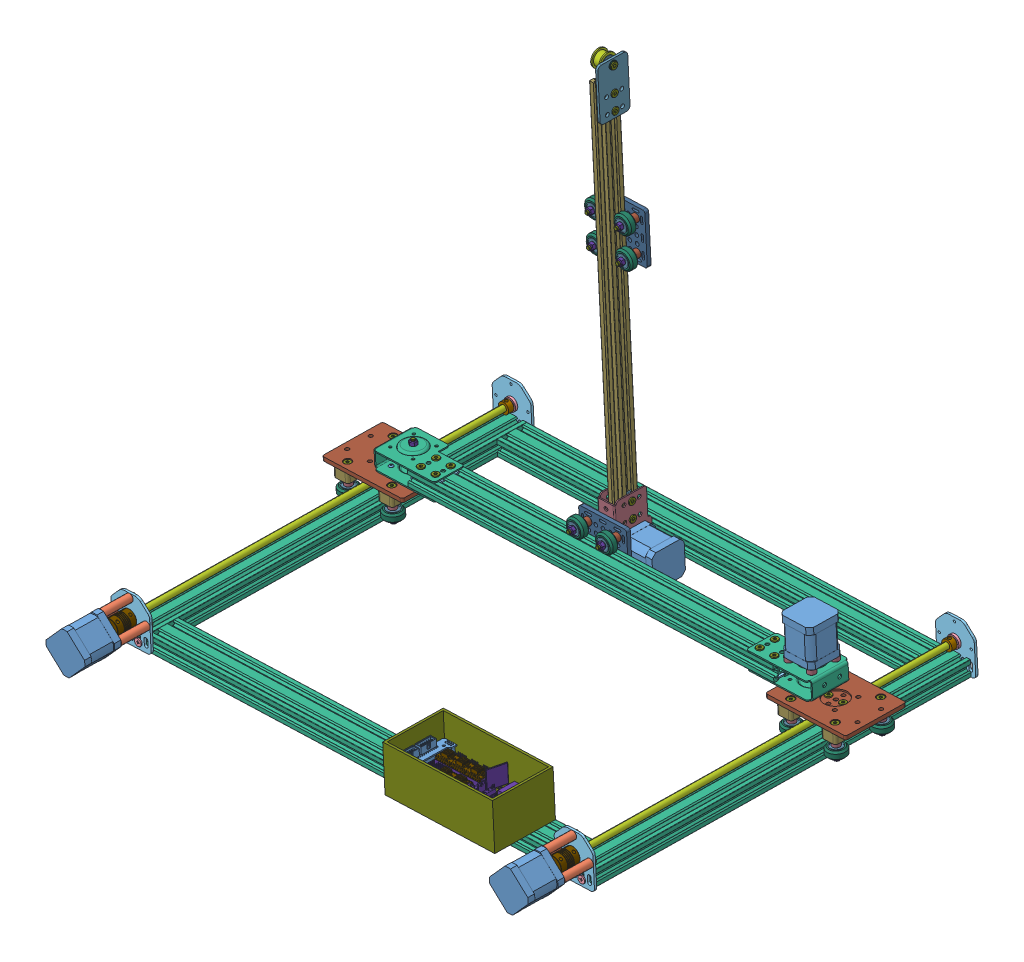
SolidWorks assembly manipulator2, configuration 預設. Lengths in mm.
Overall size (716.52 632.46 604.45).
279 component instances, 37 part files, 37 mates.
Components (placement in the parent):
- Button Head Socket Cap Screw M3-1: Button Head Socket Cap Screw M3 [M3 x 17] at (-19.1837 8.1538 443.4891) x (0.052967 -0.998596 -0.000534) z (0.000534 -0.000506 1) size (18.72 5.7 5.7)
- Button Head Socket Cap Screw M3-2: Button Head Socket Cap Screw M3 [M3 x 17] at (11.7683 9.7952 444.0184) x (0.052967 -0.998596 -0.000534) z (0.000534 -0.000506 1) size (18.72 5.7 5.7)
- Button Head Socket Cap Screw M3-3: Button Head Socket Cap Screw M3 [M3 x 17] at (-19.7114 8.1092 474.4845) x (0.052967 -0.998596 -0.000534) z (0.000534 -0.000506 1) size (18.72 5.7 5.7)
- Button Head Socket Cap Screw M3-4: Button Head Socket Cap Screw M3 [M3 x 17] at (11.2406 9.7507 475.0139) x (0.052967 -0.998596 -0.000534) z (0.000534 -0.000506 1) size (18.72 5.7 5.7)
- Nylon Insert Lock Nut M3-3: Nylon Insert Lock Nut M3 [Default] at (11.5352 14.189 444.0207) x (-0.998393 -0.052967 0.02015) z (0.02015 0.000534 0.999797) size (5.5 4 6.35)
- Nylon Insert Lock Nut M3-4: Nylon Insert Lock Nut M3 [Default] at (11.0075 14.1445 475.0162) x (-0.998393 -0.052967 0.02015) z (0.02015 0.000534 0.999797) size (5.5 4 6.35)
- Nylon Insert Lock Nut M3-5: Nylon Insert Lock Nut M3 [Default] at (-19.9445 12.503 474.4869) x (-0.998393 -0.052967 0.02015) z (0.02015 0.000534 0.999797) size (5.5 4 6.35)
- Nylon Insert Lock Nut M3-6: Nylon Insert Lock Nut M3 [Default] at (-19.4168 12.5476 443.4914) x (-0.998393 -0.052967 0.02015) z (0.02015 0.000534 0.999797) size (5.5 4 6.35)
- Aluminum Spacer 3mm-1: Aluminum Spacer 3mm [6mm] at (10.9526 25.1736 444.0266) x (0.997193 0.05292 -0.052967) z (0.052967 -0.998596 -0.000534) size (10 10 6)
- Aluminum Spacer 3mm-2: Aluminum Spacer 3mm [6mm] at (-19.9994 23.5322 443.4973) x (0.997193 0.05292 -0.052967) z (0.052967 -0.998596 -0.000534) size (10 10 6)
- Aluminum Spacer 3mm-3: Aluminum Spacer 3mm [6mm] at (-20.5271 23.4876 474.4928) x (0.997193 0.05292 -0.052967) z (0.052967 -0.998596 -0.000534) size (10 10 6)
- Aluminum Spacer 3mm-4: Aluminum Spacer 3mm [6mm] at (10.4249 25.129 475.0221) x (0.997193 0.05292 -0.052967) z (0.052967 -0.998596 -0.000534) size (10 10 6)
- Z2-1: Z2 [Default] at (-565.1545 -15.5578 336.9084) size (111.46 63.72 594.1) (flexible)
  - Ball Bearing 8 x 16 x 5-4: Ball Bearing 8 x 16 x 5 [Default] at (533.6792 21.533 -34.6863) x (-0.017023 -0.001438 0.999854) z (-0.57924 -0.815083 -0.011034) size (5 16 16)
  - Threaded Rod Plate Nema 17-3: Threaded Rod Plate Nema 17 [Default] at (533.7388 21.538 -38.1858) x (0.998451 0.05295 0.017075) z (0.052967 -0.998596 -0.000534) size (53 3 59.29)
  - V-Slot 20x40x500 Linear Rail-1: V-Slot 20x40x500 Linear Rail [Default] at (534.8758 -0.8648 -35.1982) x (0.052967 -0.998596 -0.000534) z (-0.017023 -0.001438 0.999854) size (20 40 500)
  - Threaded Rod Plate Nema 17-6: Threaded Rod Plate Nema 17 [Default] at (525.1253 20.8106 467.7404) x (-0.998451 -0.05295 -0.017075) z (0.052967 -0.998596 -0.000534) size (53 3 59.29)
  - Ball Bearing 8 x 16 x 5-6: Ball Bearing 8 x 16 x 5 [Default] at (525.1849 20.8156 464.2409) x (0.017023 0.001438 -0.999854) z (0.999854 0.001413 0.017025) size (5 16 16)
  - 8mm leadscrew 540mm-1: 8mm leadscrew 540mm [520mm] at (533.7388 21.538 -38.1858) x (-0.290929 0.956738 -0.003577) z (-0.017023 -0.001438 0.999854) size (8 8 520)
  - Shim Washer 8mm-5: Shim Washer 8mm [Default] at (525.2274 20.8192 461.7412) x (0.999711 -0.017023 0.016996) z (0.016996 0.999854 0.001727) size (11.8 1.15 11.8)
  - Shim Washer 8mm-6: Shim Washer 8mm [Default] at (533.6367 21.5294 -32.1867) x (0.99971 0.017023 0.017045) z (0.017045 -0.999854 -0.001147) size (11.8 1.15 11.8)
  - Lock Collar 8mm-5: Lock Collar 8mm [Default] at (525.3662 20.8309 453.5924) x (0.999855 -0.000012 0.017023) z (-0.017023 -0.001438 0.999854) size (14 14 7)
  - Lock Collar 8mm-6: Lock Collar 8mm [Default] at (533.6171 21.5277 -31.0369) x (0.999855 -0.000012 0.017023) z (-0.017023 -0.001438 0.999854) size (14 14 7)
  - 8mm Acme Nut Block-3: 8mm Acme Nut Block [Default] at (531.1848 21.3223 111.8263) x (-0.998451 -0.05295 -0.017075) z (-0.017023 -0.001438 0.999854) size (34 12 20)
  - mid plate-3: mid plate [預設] at (528.4577 31.3097 -5.2228) x (0.998451 0.05295 0.017075) z (-0.017023 -0.001438 0.999854) size (110 42 86.72)
    - V-Slot Gantry Plate 20-80mm 2-1: V-Slot Gantry Plate 20-80mm 2 [Default] at (4.1926 -4.0553 127) size (110 5 80)
    - Spacer Block 2-1: Spacer Block 2 [Default] at (-26.1074 -16.0553 127) x (0 0 -1) z (0 1 0) size (80 20 12)
    - Spacer Block 2-2: Spacer Block 2 [Default] at (34.4926 -16.0553 127) x (0 0 -1) z (0 1 0) size (80 20 12)
    - Aluminum Spacer 6mm-1: Aluminum Spacer 6mm [9mm] at (34.4926 -25.0553 97) x (1 0 0) z (0 1 0) size (10 10 9)
    - Aluminum Spacer 6mm-2: Aluminum Spacer 6mm [9mm] at (34.4926 -25.0553 157) x (1 0 0) z (0 1 0) size (10 10 9)
    - Aluminum Spacer 6mm-3: Aluminum Spacer 6mm [9mm] at (-26.1074 -25.0553 97) x (1 0 0) z (0 1 0) size (10 10 9)
    - Aluminum Spacer 6mm-4: Aluminum Spacer 6mm [9mm] at (-26.1074 -25.0553 157) x (1 0 0) z (0 1 0) size (10 10 9)
    - small wheel-9: small wheel [預設] at (-14.754 -38.612 99.7479) x (0 -1 0) z (0 0 1) size (11 23.9 23.9)
      - Ball Bearing 5 x 16 x 5-2: Ball Bearing 5 x 16 x 5 [Default] at (-5.0567 -11.3534 -2.7479) size (5 16 16)
      - Solid V Wheel-2: Solid V Wheel [Default] at (-8.0567 -11.3534 -2.7479) size (10.2 23.9 23.9)
      - Ball Bearing 5 x 16 x 5-3: Ball Bearing 5 x 16 x 5 [Default] at (-11.0567 -11.3534 -2.7479) size (5 16 16)
    - small wheel-10: small wheel [預設] at (-14.4269 -38.612 156.8676) x (0 -1 0) z (0.246245 0 0.969207) size (11 23.9 23.9)
      - Ball Bearing 5 x 16 x 5-2: Ball Bearing 5 x 16 x 5 [Default] at (-5.0567 -11.3534 -2.7479) size (5 16 16)
      - Solid V Wheel-2: Solid V Wheel [Default] at (-8.0567 -11.3534 -2.7479) size (10.2 23.9 23.9)
      - Ball Bearing 5 x 16 x 5-3: Ball Bearing 5 x 16 x 5 [Default] at (-11.0567 -11.3534 -2.7479) size (5 16 16)
    - small wheel-11: small wheel [預設] at (46.169 -38.612 156.6628) x (0 -1 0) z (0.263197 0 0.964742) size (11 23.9 23.9)
      - Ball Bearing 5 x 16 x 5-2: Ball Bearing 5 x 16 x 5 [Default] at (-5.0567 -11.3534 -2.7479) size (5 16 16)
      - Solid V Wheel-2: Solid V Wheel [Default] at (-8.0567 -11.3534 -2.7479) size (10.2 23.9 23.9)
      - Ball Bearing 5 x 16 x 5-3: Ball Bearing 5 x 16 x 5 [Default] at (-11.0567 -11.3534 -2.7479) size (5 16 16)
    - small wheel-12: small wheel [預設] at (45.8243 -38.612 99.8362) x (0 -1 0) z (-0.007785 0 0.99997) size (11 23.9 23.9)
      - Ball Bearing 5 x 16 x 5-2: Ball Bearing 5 x 16 x 5 [Default] at (-5.0567 -11.3534 -2.7479) size (5 16 16)
      - Solid V Wheel-2: Solid V Wheel [Default] at (-8.0567 -11.3534 -2.7479) size (10.2 23.9 23.9)
      - Ball Bearing 5 x 16 x 5-3: Ball Bearing 5 x 16 x 5 [Default] at (-11.0567 -11.3534 -2.7479) size (5 16 16)
    - Low Profile Screw M5-6: Low Profile Screw M5 [M5 x 40] at (-26.1074 -41.0553 157) x (0 -1 0) z (0 0 1) size (41.62 9 9)
    - Low Profile Screw M5-7: Low Profile Screw M5 [M5 x 40] at (-26.1074 -41.0553 97) x (0 -1 0) z (0 0 1) size (41.62 9 9)
    - Low Profile Screw M5-8: Low Profile Screw M5 [M5 x 40] at (34.4926 -41.0553 97) x (0 -1 0) z (0 0 1) size (41.62 9 9)
    - Low Profile Screw M5-10: Low Profile Screw M5 [M5 x 40] at (34.4926 -41.0553 157) x (0 -1 0) z (0 0 1) size (41.62 9 9)
    - Nylon Insert Lock Nut M5-5: Nylon Insert Lock Nut M5 [Default] at (-26.1074 -36.0553 157) x (0.837169 0 0.546944) z (0.546944 0 -0.837169) size (8 5 9.24)
    - Nylon Insert Lock Nut M5-6: Nylon Insert Lock Nut M5 [Default] at (-26.1074 -36.0553 97) x (0.837169 0 0.546944) z (0.546944 0 -0.837169) size (8 5 9.24)
    - Nylon Insert Lock Nut M5-7: Nylon Insert Lock Nut M5 [Default] at (34.4926 -36.0553 157) x (0.837169 0 0.546944) z (0.546944 0 -0.837169) size (8 5 9.24)
    - Nylon Insert Lock Nut M5-8: Nylon Insert Lock Nut M5 [Default] at (34.4926 -36.0553 97) x (0.837169 0 0.546944) z (0.546944 0 -0.837169) size (8 5 9.24)
  - Flexible Coupling 5mm x 8mm-4: Flexible Coupling 5mm x 8mm [Default] at (524.6742 20.7725 494.2365) x (-0.433195 0.90128 -0.006079) z (-0.017023 -0.001438 0.999854) size (21.03 20 25)
  - Nema 17 Stepper Motor-3: Nema 17 Stepper Motor [Default] at (524.4784 20.7559 505.7348) x (-0.743465 0.668673 -0.011696) z (0.017023 0.001438 -0.999854) size (42.42 42.42 72)
  - Aluminum Spacer 40mm-5: Aluminum Spacer 40mm [38] at (546.3648 21.9166 506.1091) x (-0.985691 -0.1677 -0.017023) z (0.017023 0.001438 -0.999854) size (10 10 38)
  - Aluminum Spacer 40mm-6: Aluminum Spacer 40mm [38] at (523.3174 42.6455 505.7465) x (-0.985691 -0.1677 -0.017023) z (0.017023 0.001438 -0.999854) size (10 10 38)
  - Aluminum Spacer 40mm-7: Aluminum Spacer 40mm [38] at (502.5921 19.5953 505.3605) x (-0.985691 -0.1677 -0.017023) z (0.017023 0.001438 -0.999854) size (10 10 38)
  - Socket Head Cap Screw M3-8: Socket Head Cap Screw M3 [M3 x 45] at (523.2493 42.6397 509.7459) x (-0.017023 -0.001438 0.999854) z (-0.999854 0.001462 -0.017021) size (48.09 5.5 5.5)
  - Socket Head Cap Screw M3-9: Socket Head Cap Screw M3 [M3 x 45] at (502.524 19.5895 509.3599) x (-0.017023 -0.001438 0.999854) z (-0.999854 0.001462 -0.017021) size (48.09 5.5 5.5)
  - Socket Head Cap Screw M3-10: Socket Head Cap Screw M3 [M3 x 45] at (546.2967 21.9109 510.1085) x (-0.017023 -0.001438 0.999854) z (-0.999854 0.001462 -0.017021) size (48.09 5.5 5.5)
  - Self Tapping Screw-1: Self Tapping Screw [Default] at (536.371 -2.4365 467.8984) x (0.99971 0.017023 0.017045) z (0.017045 -0.999854 -0.001147) size (9.6 20.4 9.6)
  - Self Tapping Screw-2: Self Tapping Screw [Default] at (516.4019 -3.4955 467.5569) x (0.99971 0.017023 0.017045) z (0.017045 -0.999854 -0.001147) size (9.6 20.4 9.6)
  - Self Tapping Screw-3: Self Tapping Screw [Default] at (544.9844 -1.7091 -38.0278) x (0.999711 -0.017023 0.016996) z (0.016996 0.999854 0.001727) size (9.6 20.4 9.6)
  - Self Tapping Screw-4: Self Tapping Screw [Default] at (525.0154 -2.7681 -38.3693) x (0.999711 -0.017023 0.016996) z (0.016996 0.999854 0.001727) size (9.6 20.4 9.6)
  - Nylon Insert Lock Nut M5-1: Nylon Insert Lock Nut M5 [Default] at (541.0521 20.8388 121.9951) x (-0.998393 -0.052967 0.02015) z (0.02015 0.000534 0.999797) size (8 5 9.24)
  - Nylon Insert Lock Nut M5-2: Nylon Insert Lock Nut M5 [Default] at (521.083 19.7798 121.6536) x (-0.998393 -0.052967 0.02015) z (0.02015 0.000534 0.999797) size (8 5 9.24)
  - Low Profile Screw M5-1: Low Profile Screw M5 [M5 x 15] at (541.3169 15.8459 121.9924) x (0.052967 -0.998596 -0.000534) z (0.000534 -0.000506 1) size (16.62 9 9)
  - Low Profile Screw M5-2: Low Profile Screw M5 [M5 x 15] at (521.3479 14.7869 121.6509) x (0.052967 -0.998596 -0.000534) z (0.000534 -0.000506 1) size (16.62 9 9)
- V-Slot 20x40x500 Linear Rail-1: V-Slot 20x40x500 Linear Rail [20 x 40 x 566] at (554.3834 14.5723 331.7116) x (-0.052967 0.998596 0.000534) z (-0.998451 -0.05295 -0.017075) size (20 40 565.91)
- V-Slot 20x40x500 Linear Rail-2: V-Slot 20x40x500 Linear Rail [20 x 40 x 566] at (546.5529 13.911 791.6445) x (-0.052967 0.998596 0.000534) z (-0.998451 -0.05295 -0.017075) size (20 40 565.91)
- Z2-4: Z2 [Default] at (39.9069 16.5297 347.2558) size (111.46 63.72 594.1) (flexible)
  - Ball Bearing 8 x 16 x 5-4: Ball Bearing 8 x 16 x 5 [Default] at (533.6792 21.533 -34.6863) x (-0.017023 -0.001438 0.999854) z (-0.57924 -0.815083 -0.011034) size (5 16 16)
  - Threaded Rod Plate Nema 17-3: Threaded Rod Plate Nema 17 [Default] at (533.7388 21.538 -38.1858) x (0.998451 0.05295 0.017075) z (0.052967 -0.998596 -0.000534) size (53 3 59.29)
  - V-Slot 20x40x500 Linear Rail-1: V-Slot 20x40x500 Linear Rail [Default] at (534.8758 -0.8648 -35.1982) x (0.052967 -0.998596 -0.000534) z (-0.017023 -0.001438 0.999854) size (20 40 500)
  - Threaded Rod Plate Nema 17-6: Threaded Rod Plate Nema 17 [Default] at (525.1253 20.8106 467.7404) x (-0.998451 -0.05295 -0.017075) z (0.052967 -0.998596 -0.000534) size (53 3 59.29)
  - Ball Bearing 8 x 16 x 5-6: Ball Bearing 8 x 16 x 5 [Default] at (525.1849 20.8156 464.2409) x (0.017023 0.001438 -0.999854) z (0.999854 0.001413 0.017025) size (5 16 16)
  - 8mm leadscrew 540mm-1: 8mm leadscrew 540mm [520mm] at (533.7388 21.538 -38.1858) x (-0.290929 0.956738 -0.003577) z (-0.017023 -0.001438 0.999854) size (8 8 520)
  - Shim Washer 8mm-5: Shim Washer 8mm [Default] at (525.2274 20.8192 461.7412) x (0.999711 -0.017023 0.016996) z (0.016996 0.999854 0.001727) size (11.8 1.15 11.8)
  - Shim Washer 8mm-6: Shim Washer 8mm [Default] at (533.6367 21.5294 -32.1867) x (0.99971 0.017023 0.017045) z (0.017045 -0.999854 -0.001147) size (11.8 1.15 11.8)
  - Lock Collar 8mm-5: Lock Collar 8mm [Default] at (525.3662 20.8309 453.5924) x (0.999855 -0.000012 0.017023) z (-0.017023 -0.001438 0.999854) size (14 14 7)
  - Lock Collar 8mm-6: Lock Collar 8mm [Default] at (533.6171 21.5277 -31.0369) x (0.999855 -0.000012 0.017023) z (-0.017023 -0.001438 0.999854) size (14 14 7)
  - 8mm Acme Nut Block-3: 8mm Acme Nut Block [Default] at (531.1848 21.3223 111.8263) x (-0.998451 -0.05295 -0.017075) z (-0.017023 -0.001438 0.999854) size (34 12 20)
  - mid plate-3: mid plate [預設] at (528.4577 31.3097 -5.2228) x (0.998451 0.05295 0.017075) z (-0.017023 -0.001438 0.999854) size (110 42 86.72)
    - V-Slot Gantry Plate 20-80mm 2-1: V-Slot Gantry Plate 20-80mm 2 [Default] at (4.1926 -4.0553 127) size (110 5 80)
    - Spacer Block 2-1: Spacer Block 2 [Default] at (-26.1074 -16.0553 127) x (0 0 -1) z (0 1 0) size (80 20 12)
    - Spacer Block 2-2: Spacer Block 2 [Default] at (34.4926 -16.0553 127) x (0 0 -1) z (0 1 0) size (80 20 12)
    - Aluminum Spacer 6mm-1: Aluminum Spacer 6mm [9mm] at (34.4926 -25.0553 97) x (1 0 0) z (0 1 0) size (10 10 9)
    - Aluminum Spacer 6mm-2: Aluminum Spacer 6mm [9mm] at (34.4926 -25.0553 157) x (1 0 0) z (0 1 0) size (10 10 9)
    - Aluminum Spacer 6mm-3: Aluminum Spacer 6mm [9mm] at (-26.1074 -25.0553 97) x (1 0 0) z (0 1 0) size (10 10 9)
    - Aluminum Spacer 6mm-4: Aluminum Spacer 6mm [9mm] at (-26.1074 -25.0553 157) x (1 0 0) z (0 1 0) size (10 10 9)
    - small wheel-9: small wheel [預設] at (-14.754 -38.612 99.7479) x (0 -1 0) z (0 0 1) size (11 23.9 23.9)
      - Ball Bearing 5 x 16 x 5-2: Ball Bearing 5 x 16 x 5 [Default] at (-5.0567 -11.3534 -2.7479) size (5 16 16)
      - Solid V Wheel-2: Solid V Wheel [Default] at (-8.0567 -11.3534 -2.7479) size (10.2 23.9 23.9)
      - Ball Bearing 5 x 16 x 5-3: Ball Bearing 5 x 16 x 5 [Default] at (-11.0567 -11.3534 -2.7479) size (5 16 16)
    - small wheel-10: small wheel [預設] at (-14.4269 -38.612 156.8676) x (0 -1 0) z (0.246245 0 0.969207) size (11 23.9 23.9)
      - Ball Bearing 5 x 16 x 5-2: Ball Bearing 5 x 16 x 5 [Default] at (-5.0567 -11.3534 -2.7479) size (5 16 16)
      - Solid V Wheel-2: Solid V Wheel [Default] at (-8.0567 -11.3534 -2.7479) size (10.2 23.9 23.9)
      - Ball Bearing 5 x 16 x 5-3: Ball Bearing 5 x 16 x 5 [Default] at (-11.0567 -11.3534 -2.7479) size (5 16 16)
    - small wheel-11: small wheel [預設] at (46.169 -38.612 156.6628) x (0 -1 0) z (0.263197 0 0.964742) size (11 23.9 23.9)
      - Ball Bearing 5 x 16 x 5-2: Ball Bearing 5 x 16 x 5 [Default] at (-5.0567 -11.3534 -2.7479) size (5 16 16)
      - Solid V Wheel-2: Solid V Wheel [Default] at (-8.0567 -11.3534 -2.7479) size (10.2 23.9 23.9)
      - Ball Bearing 5 x 16 x 5-3: Ball Bearing 5 x 16 x 5 [Default] at (-11.0567 -11.3534 -2.7479) size (5 16 16)
    - small wheel-12: small wheel [預設] at (45.8243 -38.612 99.8362) x (0 -1 0) z (-0.007785 0 0.99997) size (11 23.9 23.9)
      - Ball Bearing 5 x 16 x 5-2: Ball Bearing 5 x 16 x 5 [Default] at (-5.0567 -11.3534 -2.7479) size (5 16 16)
      - Solid V Wheel-2: Solid V Wheel [Default] at (-8.0567 -11.3534 -2.7479) size (10.2 23.9 23.9)
      - Ball Bearing 5 x 16 x 5-3: Ball Bearing 5 x 16 x 5 [Default] at (-11.0567 -11.3534 -2.7479) size (5 16 16)
    - Low Profile Screw M5-6: Low Profile Screw M5 [M5 x 40] at (-26.1074 -41.0553 157) x (0 -1 0) z (0 0 1) size (41.62 9 9)
    - Low Profile Screw M5-7: Low Profile Screw M5 [M5 x 40] at (-26.1074 -41.0553 97) x (0 -1 0) z (0 0 1) size (41.62 9 9)
    - Low Profile Screw M5-8: Low Profile Screw M5 [M5 x 40] at (34.4926 -41.0553 97) x (0 -1 0) z (0 0 1) size (41.62 9 9)
    - Low Profile Screw M5-10: Low Profile Screw M5 [M5 x 40] at (34.4926 -41.0553 157) x (0 -1 0) z (0 0 1) size (41.62 9 9)
    - Nylon Insert Lock Nut M5-5: Nylon Insert Lock Nut M5 [Default] at (-26.1074 -36.0553 157) x (0.837169 0 0.546944) z (0.546944 0 -0.837169) size (8 5 9.24)
    - Nylon Insert Lock Nut M5-6: Nylon Insert Lock Nut M5 [Default] at (-26.1074 -36.0553 97) x (0.837169 0 0.546944) z (0.546944 0 -0.837169) size (8 5 9.24)
    - Nylon Insert Lock Nut M5-7: Nylon Insert Lock Nut M5 [Default] at (34.4926 -36.0553 157) x (0.837169 0 0.546944) z (0.546944 0 -0.837169) size (8 5 9.24)
    - Nylon Insert Lock Nut M5-8: Nylon Insert Lock Nut M5 [Default] at (34.4926 -36.0553 97) x (0.837169 0 0.546944) z (0.546944 0 -0.837169) size (8 5 9.24)
  - Flexible Coupling 5mm x 8mm-4: Flexible Coupling 5mm x 8mm [Default] at (524.6742 20.7725 494.2365) x (-0.433195 0.90128 -0.006079) z (-0.017023 -0.001438 0.999854) size (21.03 20 25)
  - Nema 17 Stepper Motor-3: Nema 17 Stepper Motor [Default] at (524.4784 20.7559 505.7348) x (-0.743465 0.668673 -0.011696) z (0.017023 0.001438 -0.999854) size (42.42 42.42 72)
  - Aluminum Spacer 40mm-5: Aluminum Spacer 40mm [38] at (546.3648 21.9166 506.1091) x (-0.985691 -0.1677 -0.017023) z (0.017023 0.001438 -0.999854) size (10 10 38)
  - Aluminum Spacer 40mm-6: Aluminum Spacer 40mm [38] at (523.3174 42.6455 505.7465) x (-0.985691 -0.1677 -0.017023) z (0.017023 0.001438 -0.999854) size (10 10 38)
  - Aluminum Spacer 40mm-7: Aluminum Spacer 40mm [38] at (502.5921 19.5953 505.3605) x (-0.985691 -0.1677 -0.017023) z (0.017023 0.001438 -0.999854) size (10 10 38)
  - Socket Head Cap Screw M3-8: Socket Head Cap Screw M3 [M3 x 45] at (523.2493 42.6397 509.7459) x (-0.017023 -0.001438 0.999854) z (-0.999854 0.001462 -0.017021) size (48.09 5.5 5.5)
  - Socket Head Cap Screw M3-9: Socket Head Cap Screw M3 [M3 x 45] at (502.524 19.5895 509.3599) x (-0.017023 -0.001438 0.999854) z (-0.999854 0.001462 -0.017021) size (48.09 5.5 5.5)
  - Socket Head Cap Screw M3-10: Socket Head Cap Screw M3 [M3 x 45] at (546.2967 21.9109 510.1085) x (-0.017023 -0.001438 0.999854) z (-0.999854 0.001462 -0.017021) size (48.09 5.5 5.5)
  - Self Tapping Screw-1: Self Tapping Screw [Default] at (536.371 -2.4365 467.8984) x (0.99971 0.017023 0.017045) z (0.017045 -0.999854 -0.001147) size (9.6 20.4 9.6)
  - Self Tapping Screw-2: Self Tapping Screw [Default] at (516.4019 -3.4955 467.5569) x (0.99971 0.017023 0.017045) z (0.017045 -0.999854 -0.001147) size (9.6 20.4 9.6)
  - Self Tapping Screw-3: Self Tapping Screw [Default] at (544.9844 -1.7091 -38.0278) x (0.999711 -0.017023 0.016996) z (0.016996 0.999854 0.001727) size (9.6 20.4 9.6)
  - Self Tapping Screw-4: Self Tapping Screw [Default] at (525.0154 -2.7681 -38.3693) x (0.999711 -0.017023 0.016996) z (0.016996 0.999854 0.001727) size (9.6 20.4 9.6)
  - Nylon Insert Lock Nut M5-1: Nylon Insert Lock Nut M5 [Default] at (541.0521 20.8388 121.9951) x (-0.998393 -0.052967 0.02015) z (0.02015 0.000534 0.999797) size (8 5 9.24)
  - Nylon Insert Lock Nut M5-2: Nylon Insert Lock Nut M5 [Default] at (521.083 19.7798 121.6536) x (-0.998393 -0.052967 0.02015) z (0.02015 0.000534 0.999797) size (8 5 9.24)
  - Low Profile Screw M5-1: Low Profile Screw M5 [M5 x 15] at (541.3169 15.8459 121.9924) x (0.052967 -0.998596 -0.000534) z (0.000534 -0.000506 1) size (16.62 9 9)
  - Low Profile Screw M5-2: Low Profile Screw M5 [M5 x 15] at (521.3479 14.7869 121.6509) x (0.052967 -0.998596 -0.000534) z (0.000534 -0.000506 1) size (16.62 9 9)
- Y-1: Y [Default] at (-55.2828 466.9625 1561.8962) x (0.061515 -0.998106 -0.000537) z (0.998106 0.061515 -0.00018) size (96.36 65.23 599.86) (flexible)
  - Aluminum Spacer 6mm-1: Aluminum Spacer 6mm [Default] at (421.0945 1108.215 584.4034) x (0.00697 0.580866 0.813969) z (0.999963 -0.000001 -0.008562) size (10 10 6)
  - Aluminum Spacer 6mm-2: Aluminum Spacer 6mm [Default] at (427.0897 1077.2197 583.817) x (-0.008174 0.297659 -0.954637) z (-0.999963 0.000001 0.008562) size (10 10 6)
  - Aluminum Spacer 6mm-3: Aluminum Spacer 6mm [Default] at (426.8289 1108.7501 553.3578) x (-0.008322 0.234979 -0.971965) z (-0.999963 0.000001 0.008562) size (10 10 6)
  - Aluminum Spacer 6mm-4: Aluminum Spacer 6mm [Default] at (420.8245 1077.7547 552.8741) x (0.003973 0.88592 0.463821) z (0.999963 -0.000001 -0.008562) size (10 10 6)
  - Aluminum Spacer 6mm-7: Aluminum Spacer 6mm [Default] at (446.3917 1102.3933 23.3622) x (0.008562 0.000001 0.999963) z (-0.999963 0.000001 0.008562) size (10 10 6)
  - Aluminum Spacer 6mm-8: Aluminum Spacer 6mm [Default] at (427.2924 1102.3934 23.5258) x (0.00638 -0.666766 0.74524) z (-0.999963 0.000001 0.008562) size (10 10 6)
  - Button Head Socket Cap Screw M3-2: Button Head Socket Cap Screw M3 [M3 x 12] at (416.6947 1108.2151 584.4411) x (-0.999963 0.000001 0.008562) z (0.003271 0.924225 0.381835) size (13.72 5.7 5.7)
  - Button Head Socket Cap Screw M3-4: Button Head Socket Cap Screw M3 [M3 x 12] at (416.4247 1077.7547 552.9118) x (-0.999963 0.000001 0.008562) z (0.003271 0.924225 0.381835) size (13.72 5.7 5.7)
  - Button Head Socket Cap Screw M3-5: Button Head Socket Cap Screw M3 [M3 x 12] at (416.6901 1077.2197 583.906) x (-0.999963 0.000001 0.008562) z (0.003271 0.924225 0.381835) size (13.72 5.7 5.7)
  - Double Tee Nut-9: Double Tee Nut [Default] at (446.246 1069.0645 508.5583) x (0.008561 -0.01726 0.999814) z (-0.999963 0.000001 0.008562) size (36.88 10 3)
  - Double Tee Nut-14: Double Tee Nut [Default] at (446.249 1089.0615 508.9035) x (0.008561 -0.01726 0.999814) z (-0.999963 0.000001 0.008562) size (36.88 10 3)
  - Double Tee Nut-15: Double Tee Nut [Default] at (430.1623 1068.428 545.5719) x (-0.008561 0.01726 -0.999814) z (0.999963 -0.000001 -0.008562) size (36.88 10 3)
  - Double Tee Nut-16: Double Tee Nut [Default] at (430.1653 1088.425 545.917) x (-0.008561 0.01726 -0.999814) z (0.999963 -0.000001 -0.008562) size (36.88 10 3)
  - Double Tee Nut-20: Double Tee Nut [Default] at (426.2006 1096.4182 82.883) x (-0.008561 0.01726 -0.999814) z (0.999963 -0.000001 -0.008562) size (36.88 10 3)
  - Double Tee Nut-19: Double Tee Nut [Default] at (426.1976 1076.4212 82.5378) x (-0.008561 0.01726 -0.999814) z (0.999963 -0.000001 -0.008562) size (36.88 10 3)
  - Double Tee Nut-21: Double Tee Nut [Default] at (442.2842 1097.0547 45.8694) x (0.008561 -0.01726 0.999814) z (-0.999963 0.000001 0.008562) size (36.88 10 3)
  - Double Tee Nut-22: Double Tee Nut [Default] at (442.2813 1077.0577 45.5242) x (0.008561 -0.01726 0.999814) z (-0.999963 0.000001 0.008562) size (36.88 10 3)
  - Low Profile Screw M5-18: Low Profile Screw M5 [M5 x 6] at (428.729 1101.5631 74.5086) x (0.999963 -0.000001 -0.008562) z (0.003416 0.917023 0.398819) size (7.62 9 9)
  - Low Profile Screw M5-19: Low Profile Screw M5 [M5 x 6] at (428.726 1081.5661 74.1634) x (0.999963 -0.000001 -0.008562) z (0.006235 -0.685246 0.728285) size (7.62 9 9)
  - Low Profile Screw M5-20: Low Profile Screw M5 [M5 x 6] at (428.5548 1081.9113 54.1671) x (0.999963 -0.000001 -0.008562) z (-0.004605 -0.843137 -0.537678) size (7.62 9 9)
  - Low Profile Screw M5-21: Low Profile Screw M5 [M5 x 6] at (428.5577 1101.9083 54.5123) x (0.999963 -0.000001 -0.008562) z (-0.001108 -0.991612 -0.129244) size (7.62 9 9)
  - Low Profile Screw M5-22: Low Profile Screw M5 [M5 x 6] at (439.9285 1101.5631 74.4127) x (-0.999963 0.000001 0.008562) z (-0.008562 -0.000275 -0.999963) size (7.62 9 9)
  - Low Profile Screw M5-23: Low Profile Screw M5 [M5 x 6] at (439.7573 1101.9083 54.4164) x (-0.999963 0.000001 0.008562) z (-0.008562 -0.000275 -0.999963) size (7.62 9 9)
  - Low Profile Screw M5-24: Low Profile Screw M5 [M5 x 6] at (439.9256 1081.5661 74.0675) x (-0.999963 0.000001 0.008562) z (-0.008562 -0.000275 -0.999963) size (7.62 9 9)
  - Low Profile Screw M5-25: Low Profile Screw M5 [M5 x 6] at (439.7543 1081.9113 54.0712) x (-0.999963 0.000001 0.008562) z (-0.008562 -0.000275 -0.999963) size (7.62 9 9)
  - Low Profile Screw M5-26: Low Profile Screw M5 [M5 x 6] at (432.6937 1093.5699 537.5426) x (0.999963 -0.000001 -0.008562) z (0.008562 0 0.999963) size (7.62 9 9)
  - Low Profile Screw M5-28: Low Profile Screw M5 [M5 x 6] at (432.5195 1073.9181 517.2012) x (0.999963 -0.000001 -0.008562) z (0.008562 0 0.999963) size (7.62 9 9)
  - Low Profile Screw M5-29: Low Profile Screw M5 [M5 x 6] at (432.6907 1073.5729 537.1975) x (0.999963 -0.000001 -0.008562) z (0.008562 0 0.999963) size (7.62 9 9)
  - Low Profile Screw M5-30: Low Profile Screw M5 [M5 x 6] at (443.8933 1093.5699 537.4467) x (-0.999963 0.000001 0.008562) z (-0.006172 0.693056 -0.720857) size (7.62 9 9)
  - Low Profile Screw M5-31: Low Profile Screw M5 [M5 x 6] at (443.7221 1093.9151 517.4504) x (-0.999963 0.000001 0.008562) z (-0.007544 -0.473064 -0.880996) size (7.62 9 9)
  - Low Profile Screw M5-32: Low Profile Screw M5 [M5 x 6] at (443.8903 1073.5729 537.1016) x (-0.999963 0.000001 0.008562) z (-0.008393 -0.198144 -0.980137) size (7.62 9 9)
  - Low Profile Screw M5-33: Low Profile Screw M5 [M5 x 6] at (443.7191 1073.9181 517.1053) x (-0.999963 0.000001 0.008562) z (-0.005369 0.778884 -0.627145) size (7.62 9 9)
  - Low Profile Screw M5-34: Low Profile Screw M5 [M5 x 35] at (413.0929 1102.3934 23.6473) x (-0.999963 0.000001 0.008562) z (-0.007276 0.527011 -0.849827) size (36.62 9 9)
  - Nylon Insert Lock Nut M5-2: Nylon Insert Lock Nut M5 [Default] at (419.6927 1102.3934 23.5908) x (0.004535 0.848273 0.529539) z (0.007263 -0.529559 0.848242) size (8 5 9.24)
  - Low Profile Screw M5-35: Low Profile Screw M5 [M5 x 6] at (432.5225 1093.9151 517.5463) x (0.999963 -0.000001 -0.008562) z (0.008562 0 0.999963) size (7.62 9 9)
  - Button Head Socket Cap Screw M3-25: Button Head Socket Cap Screw M3 [M3 x 12] at (416.4293 1108.7501 553.4468) x (-0.999963 0.000001 0.008562) z (-0.008562 -0.000275 -0.999963) size (13.72 5.7 5.7)
  - Linear Actuator End Mount-1: Linear Actuator End Mount [Default] at (438.7777 1019.7292 594.0567) x (-0.999963 0.000001 0.008562) z (-0.008561 0.01726 -0.999814) size (28.4 54.9 86.33)
  - Linear Actuator End Mount-2: Linear Actuator End Mount [Default] at (433.6516 1030.0638 -4.6124) x (0.999963 -0.000001 -0.008562) z (0.008561 -0.01726 0.999814) size (28.4 54.9 86.33)
  - Nema 17 Stepper Motor-1: Nema 17 Stepper Motor [Default] at (420.9595 1092.9849 568.6388) x (-0.008561 0.01726 -0.999814) z (0.999963 -0.000001 -0.008562) size (42.42 42.42 72)
  - Smooth Idler-1: Smooth Idler [Default] at (433.8421 1102.3934 23.4697) x (0.999963 -0.000001 -0.008562) z (0.005218 -0.7928 0.609459) size (13.1 22 22)
    - Smooth Idler Pulley Wheel-1: Smooth Idler Pulley Wheel [Default] at origin size (12.7 22 22)
    - Ball Bearing 5 x 16 x 5-1: Ball Bearing 5 x 16 x 5 [Default] at (4.05 0 0) x (1 0 0) z (0 0.954651 0.297727) size (5 16 16)
    - Ball Bearing 5 x 16 x 5-2: Ball Bearing 5 x 16 x 5 [Default] at (-4.05 0 0) x (1 0 0) z (0 0.976216 -0.216802) size (5 16 16)
    - Nylon Spacer 0.125in-1: Nylon Spacer 0.125in [Default] at (-1.625 0 0) x (0 -0.24187 -0.970309) z (0 -0.970309 0.24187) size (7.94 3.17 7.94)
  - GT2 Timing Pulley 30 Tooth-1: GT2 Timing Pulley 30 Tooth [Default] at (426.6593 1092.9849 568.59) x (0.999963 -0.000001 -0.008562) z (-0.007129 -0.55389 -0.832559) size (17.5 22 22)
  - V-Slot 20x40x500 Linear Rail-1: V-Slot 20x40x500 Linear Rail [Default] at (434.0838 1092.0555 45.8533) x (0.999963 -0.000001 -0.008562) z (0.008561 -0.01726 0.999814) size (20 40 500)
  - small plate-2: small plate [預設] at (444.4195 1082.4526 226.1786) x (0.999761 -0.019668 -0.009529) z (0.009662 0.00665 0.999931) size (65.63 34.48 65.67)
    - small wheel-3: small wheel [預設] at (-0.7158 22.993 64.759) x (-0.019681 0.99952 0.023908) z (0.000235 -0.023908 0.999714) size (11 23.9 23.9)
      - Ball Bearing 5 x 16 x 5-2: Ball Bearing 5 x 16 x 5 [Default] at (-5.0567 -11.3534 -2.7479) size (5 16 16)
      - Solid V Wheel-2: Solid V Wheel [Default] at (-8.0567 -11.3534 -2.7479) size (10.2 23.9 23.9)
      - Ball Bearing 5 x 16 x 5-3: Ball Bearing 5 x 16 x 5 [Default] at (-11.0567 -11.3534 -2.7479) size (5 16 16)
    - small wheel-4: small wheel [預設] at (-40.708 22.2066 64.715) x (-0.019681 0.99952 0.023908) z (0.000235 -0.023908 0.999714) size (11 23.9 23.9)
      - Ball Bearing 5 x 16 x 5-2: Ball Bearing 5 x 16 x 5 [Default] at (-5.0567 -11.3534 -2.7479) size (5 16 16)
      - Solid V Wheel-2: Solid V Wheel [Default] at (-8.0567 -11.3534 -2.7479) size (10.2 23.9 23.9)
      - Ball Bearing 5 x 16 x 5-3: Ball Bearing 5 x 16 x 5 [Default] at (-11.0567 -11.3534 -2.7479) size (5 16 16)
    - V-Slot Gantry Plate 20mm 2-1: V-Slot Gantry Plate 20mm 2 [Default] at (-9.4756 29.8077 42.1523) x (0.999806 0.01966 0.0011) z (-0.000629 -0.023925 0.999714) size (65.5 5 65.5)
    - small wheel-5: small wheel [預設] at (-0.6906 23.95 24.7704) x (-0.019681 0.99952 0.023908) z (0.000235 -0.023908 0.999714) size (11 23.9 23.9)
